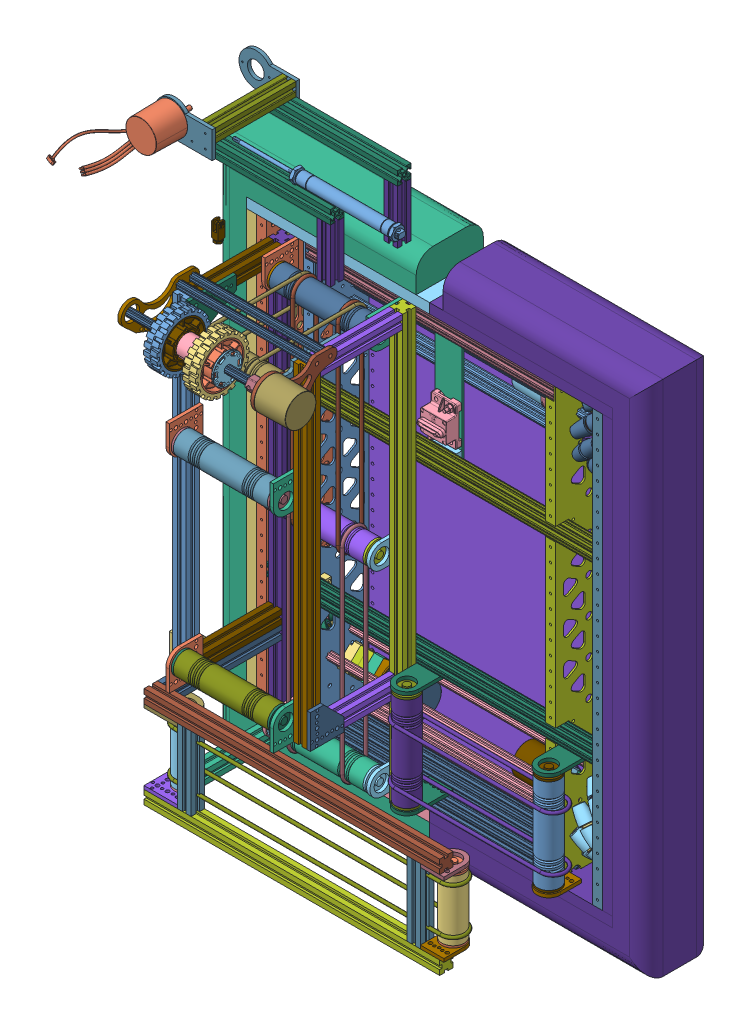
SolidWorks assembly Robot 2020, configuration Default. Lengths in mm. (continued)
Components (placement in the parent): (continued)
- Robot 2020(2)^Robot 2020-1: Robot 2020(2)^Robot 2020 [Default] at origin size (819.15 992.53 549) (virtual) (continued)
  - Fame 2020^Robot 2020(2)_Robot 2020-1: Fame 2020^Robot 2020(2)_Robot 2020 [Default] at origin size (819.15 977.9 171.99) (virtual) (continued)
    - Left Wheel Assembly v4(Mirror) (2)^Fame 2020_Robot 2020(2)_Robot 2020-1: Left Wheel Assembly v4(Mirror) (2)^Fame 2020_Robot 2020(2)_Robot 2020 [Default] at (500 0 0) x (1 0 0) z (0 0 -1) size (65.82 166.11 165.01) (virtual) (continued)
      - 6_Mecanum_Wheel_Left_217-2799 v1(Mirror) (2)^Left Wheel Assembly v4(Mirror) (2)_Fame 2020_Robot 2020(2)_Robot 2020-1: 6_Mecanum_Wheel_Left_217-2799 v1(Mirror) (2)^Left Wheel Assembly v4(Mirror) (2)_Fame 2020_Robot 2020(2)_Robot 2020 [Default] x (0 0 -1) z (1 0 0) size (165.01 166.11 65.82) (virtual) (continued)
        - 217-2586-007 Rev1(Mirror) (2)^6_Mecanum_Wheel_Left_217-2799 v1(Mirror) (2)_Left Wheel Assembly v4(Mirror) (2)_Fame 2020_Robot 2020(2)_Robot 2020-10: 217-2586-007 Rev1(Mirror) (2)^6_Mecanum_Wheel_Left_217-2799 v1(Mirror) (2)_Left Wheel Assembly v4(Mirror) (2)_Fame 2020_Robot 2020(2)_Robot 2020 [Default] at (23.6484 -378.9904 -227.6598) x (0.698401 -0.110616 -0.707107) z (0.159162 0.987249 0.002763) size (61.72 5 5) (virtual)
        - 217-2586-008 Rev1(Mirror) (2)^6_Mecanum_Wheel_Left_217-2799 v1(Mirror) (2)_Left Wheel Assembly v4(Mirror) (2)_Fame 2020_Robot 2020(2)_Robot 2020-1: 217-2586-008 Rev1(Mirror) (2)^6_Mecanum_Wheel_Left_217-2799 v1(Mirror) (2)_Left Wheel Assembly v4(Mirror) (2)_Fame 2020_Robot 2020(2)_Robot 2020 [Default] at (53.3583 -330.4692 -227.5328) x (0.544639 0.838671 0) z (0 0 -1) size (7.33 6.35 31.75) (virtual)
        - 217-2586-008 Rev1(Mirror) (2)^6_Mecanum_Wheel_Left_217-2799 v1(Mirror) (2)_Left Wheel Assembly v4(Mirror) (2)_Fame 2020_Robot 2020(2)_Robot 2020-2: 217-2586-008 Rev1(Mirror) (2)^6_Mecanum_Wheel_Left_217-2799 v1(Mirror) (2)_Left Wheel Assembly v4(Mirror) (2)_Fame 2020_Robot 2020(2)_Robot 2020 [Default] at (32.1413 -341.2799 -227.5328) x (0.99863 -0.052336 0) z (0 0 -1) size (7.33 6.35 31.75) (virtual)
        - 217-2586-008 Rev1(Mirror) (2)^6_Mecanum_Wheel_Left_217-2799 v1(Mirror) (2)_Left Wheel Assembly v4(Mirror) (2)_Fame 2020_Robot 2020(2)_Robot 2020-3: 217-2586-008 Rev1(Mirror) (2)^6_Mecanum_Wheel_Left_217-2799 v1(Mirror) (2)_Left Wheel Assembly v4(Mirror) (2)_Fame 2020_Robot 2020(2)_Robot 2020 [Default] at (12.1704 -328.3106 -227.5328) x (0.45399 -0.891007 0) z (0 0 -1) size (7.33 6.35 31.75) (virtual)
        - 217-2586-008 Rev1(Mirror) (2)^6_Mecanum_Wheel_Left_217-2799 v1(Mirror) (2)_Left Wheel Assembly v4(Mirror) (2)_Fame 2020_Robot 2020(2)_Robot 2020-4: 217-2586-008 Rev1(Mirror) (2)^6_Mecanum_Wheel_Left_217-2799 v1(Mirror) (2)_Left Wheel Assembly v4(Mirror) (2)_Fame 2020_Robot 2020(2)_Robot 2020 [Default] at (13.4167 -304.5308 -227.5328) x (-0.544639 -0.838671 0) z (0 0 -1) size (7.33 6.35 31.75) (virtual)
        - 217-2586-008 Rev1(Mirror) (2)^6_Mecanum_Wheel_Left_217-2799 v1(Mirror) (2)_Left Wheel Assembly v4(Mirror) (2)_Fame 2020_Robot 2020(2)_Robot 2020-5: 217-2586-008 Rev1(Mirror) (2)^6_Mecanum_Wheel_Left_217-2799 v1(Mirror) (2)_Left Wheel Assembly v4(Mirror) (2)_Fame 2020_Robot 2020(2)_Robot 2020 [Default] at (34.6337 -293.7201 -227.5328) x (-0.99863 0.052336 0) z (0 0 -1) size (7.33 6.35 31.75) (virtual)
        - 217-2586-008 Rev1(Mirror) (2)^6_Mecanum_Wheel_Left_217-2799 v1(Mirror) (2)_Left Wheel Assembly v4(Mirror) (2)_Fame 2020_Robot 2020(2)_Robot 2020-6: 217-2586-008 Rev1(Mirror) (2)^6_Mecanum_Wheel_Left_217-2799 v1(Mirror) (2)_Left Wheel Assembly v4(Mirror) (2)_Fame 2020_Robot 2020(2)_Robot 2020 [Default] at (54.6046 -306.6894 -227.5328) x (-0.45399 0.891007 0) z (0 0 -1) size (7.33 6.35 31.75) (virtual)
        - NUT-832-NYLOCK(Mirror) (2)^6_Mecanum_Wheel_Left_217-2799 v1(Mirror) (2)_Left Wheel Assembly v4(Mirror) (2)_Fame 2020_Robot 2020(2)_Robot 2020-1: NUT-832-NYLOCK(Mirror) (2)^6_Mecanum_Wheel_Left_217-2799 v1(Mirror) (2)_Left Wheel Assembly v4(Mirror) (2)_Fame 2020_Robot 2020(2)_Robot 2020 [Default] at (6.1639 -290.2764 -241.3161) x (0.258819 -0.965926 0) z (0.965926 0.258819 0) size (9.37 5.86 8.12) (virtual)
        - NUT-832-NYLOCK(Mirror) (2)^6_Mecanum_Wheel_Left_217-2799 v1(Mirror) (2)_Left Wheel Assembly v4(Mirror) (2)_Fame 2020_Robot 2020(2)_Robot 2020-2: NUT-832-NYLOCK(Mirror) (2)^6_Mecanum_Wheel_Left_217-2799 v1(Mirror) (2)_Left Wheel Assembly v4(Mirror) (2)_Fame 2020_Robot 2020(2)_Robot 2020 [Default] at (-0.9163 -334.9786 -241.3161) x (0.99863 -0.052336 0) z (0.052336 0.99863 0) size (9.37 5.86 8.12) (virtual)
        - NUT-832-NYLOCK(Mirror) (2)^6_Mecanum_Wheel_Left_217-2799 v1(Mirror) (2)_Left Wheel Assembly v4(Mirror) (2)_Fame 2020_Robot 2020(2)_Robot 2020-3: NUT-832-NYLOCK(Mirror) (2)^6_Mecanum_Wheel_Left_217-2799 v1(Mirror) (2)_Left Wheel Assembly v4(Mirror) (2)_Fame 2020_Robot 2020(2)_Robot 2020 [Default] at (39.4102 -355.526 -241.3161) x (0.358368 0.93358 0) z (-0.93358 0.358368 0) size (9.37 5.86 8.12) (virtual)
        - NUT-832-NYLOCK(Mirror) (2)^6_Mecanum_Wheel_Left_217-2799 v1(Mirror) (2)_Left Wheel Assembly v4(Mirror) (2)_Fame 2020_Robot 2020(2)_Robot 2020-4: NUT-832-NYLOCK(Mirror) (2)^6_Mecanum_Wheel_Left_217-2799 v1(Mirror) (2)_Left Wheel Assembly v4(Mirror) (2)_Fame 2020_Robot 2020(2)_Robot 2020 [Default] at (71.4135 -323.5227 -241.3161) x (-0.777146 0.62932 0) z (-0.62932 -0.777146 0) size (9.37 5.86 8.12) (virtual)
        - NUT-832-NYLOCK(Mirror) (2)^6_Mecanum_Wheel_Left_217-2799 v1(Mirror) (2)_Left Wheel Assembly v4(Mirror) (2)_Fame 2020_Robot 2020(2)_Robot 2020-5: NUT-832-NYLOCK(Mirror) (2)^6_Mecanum_Wheel_Left_217-2799 v1(Mirror) (2)_Left Wheel Assembly v4(Mirror) (2)_Fame 2020_Robot 2020(2)_Robot 2020 [Default] at (50.8661 -283.1962 -241.3161) x (-0.838671 -0.544639 0) z (0.544639 -0.838671 0) size (9.37 5.86 8.12) (virtual)
        - SCREW-832-1250(Mirror) (2)^6_Mecanum_Wheel_Left_217-2799 v1(Mirror) (2)_Left Wheel Assembly v4(Mirror) (2)_Fame 2020_Robot 2020(2)_Robot 2020-1: SCREW-832-1250(Mirror) (2)^6_Mecanum_Wheel_Left_217-2799 v1(Mirror) (2)_Left Wheel Assembly v4(Mirror) (2)_Fame 2020_Robot 2020(2)_Robot 2020 [Default] at (6.1639 -290.2764 -212.75) x (0 0 -1) z (0.394243 -0.919006 0) size (33.96 7.92 7.92) (virtual)
        - SCREW-832-1250(Mirror) (2)^6_Mecanum_Wheel_Left_217-2799 v1(Mirror) (2)_Left Wheel Assembly v4(Mirror) (2)_Fame 2020_Robot 2020(2)_Robot 2020-2: SCREW-832-1250(Mirror) (2)^6_Mecanum_Wheel_Left_217-2799 v1(Mirror) (2)_Left Wheel Assembly v4(Mirror) (2)_Fame 2020_Robot 2020(2)_Robot 2020 [Default] at (-0.9163 -334.9786 -212.75) x (0 0 -1) z (0.995855 0.090959 0) size (33.96 7.92 7.92) (virtual)
        - SCREW-832-1250(Mirror) (2)^6_Mecanum_Wheel_Left_217-2799 v1(Mirror) (2)_Left Wheel Assembly v4(Mirror) (2)_Fame 2020_Robot 2020(2)_Robot 2020-3: SCREW-832-1250(Mirror) (2)^6_Mecanum_Wheel_Left_217-2799 v1(Mirror) (2)_Left Wheel Assembly v4(Mirror) (2)_Fame 2020_Robot 2020(2)_Robot 2020 [Default] at (39.4102 -355.526 -212.75) x (0 0 -1) z (0.221229 0.975222 0) size (33.96 7.92 7.92) (virtual)
        - SCREW-832-1250(Mirror) (2)^6_Mecanum_Wheel_Left_217-2799 v1(Mirror) (2)_Left Wheel Assembly v4(Mirror) (2)_Fame 2020_Robot 2020(2)_Robot 2020-4: SCREW-832-1250(Mirror) (2)^6_Mecanum_Wheel_Left_217-2799 v1(Mirror) (2)_Left Wheel Assembly v4(Mirror) (2)_Fame 2020_Robot 2020(2)_Robot 2020 [Default] at (71.4135 -323.5227 -212.75) x (0 0 -1) z (-0.859128 0.511761 0) size (33.96 7.92 7.92) (virtual)
        - SCREW-832-1250(Mirror) (2)^6_Mecanum_Wheel_Left_217-2799 v1(Mirror) (2)_Left Wheel Assembly v4(Mirror) (2)_Fame 2020_Robot 2020(2)_Robot 2020-5: SCREW-832-1250(Mirror) (2)^6_Mecanum_Wheel_Left_217-2799 v1(Mirror) (2)_Left Wheel Assembly v4(Mirror) (2)_Fame 2020_Robot 2020(2)_Robot 2020 [Default] at (50.8661 -283.1962 -212.75) x (0 0 -1) z (-0.752199 -0.658936 0) size (33.96 7.92 7.92) (virtual)
        - 217-2586-005 Rev2(Mirror) (2)^6_Mecanum_Wheel_Left_217-2799 v1(Mirror) (2)_Left Wheel Assembly v4(Mirror) (2)_Fame 2020_Robot 2020(2)_Robot 2020-1: 217-2586-005 Rev2(Mirror) (2)^6_Mecanum_Wheel_Left_217-2799 v1(Mirror) (2)_Left Wheel Assembly v4(Mirror) (2)_Fame 2020_Robot 2020(2)_Robot 2020 [Default] at (-6.1597 -365.9972 -233.9884) x (-0.5 0.5 0.707107) z (-0.146447 -0.853553 0.5) size (8.5 8 8) (virtual)
        - 217-2586-005 Rev2(Mirror) (2)^6_Mecanum_Wheel_Left_217-2799 v1(Mirror) (2)_Left Wheel Assembly v4(Mirror) (2)_Fame 2020_Robot 2020(2)_Robot 2020-2: 217-2586-005 Rev2(Mirror) (2)^6_Mecanum_Wheel_Left_217-2799 v1(Mirror) (2)_Left Wheel Assembly v4(Mirror) (2)_Fame 2020_Robot 2020(2)_Robot 2020 [Default] at (-15.1097 -357.0472 -221.3312) x (-0.5 0.5 0.707107) z (-0.146447 -0.853553 0.5) size (8.5 8 8) (virtual)
        - 217-2586-005 Rev2(Mirror) (2)^6_Mecanum_Wheel_Left_217-2799 v1(Mirror) (2)_Left Wheel Assembly v4(Mirror) (2)_Fame 2020_Robot 2020(2)_Robot 2020-3: 217-2586-005 Rev2(Mirror) (2)^6_Mecanum_Wheel_Left_217-2799 v1(Mirror) (2)_Left Wheel Assembly v4(Mirror) (2)_Fame 2020_Robot 2020(2)_Robot 2020 [Default] at (-29.0929 -320.9884 -221.3312) x (-0.110616 0.698401 0.707107) z (-0.620184 -0.60446 0.5) size (8.5 8 8) (virtual)
        - 217-2586-005 Rev2(Mirror) (2)^6_Mecanum_Wheel_Left_217-2799 v1(Mirror) (2)_Left Wheel Assembly v4(Mirror) (2)_Fame 2020_Robot 2020(2)_Robot 2020-4: 217-2586-005 Rev2(Mirror) (2)^6_Mecanum_Wheel_Left_217-2799 v1(Mirror) (2)_Left Wheel Assembly v4(Mirror) (2)_Fame 2020_Robot 2020(2)_Robot 2020 [Default] at (-19.2106 -283.5972 -221.3312) x (0.32102 0.630037 0.707107) z (-0.857032 -0.124484 0.5) size (8.5 8 8) (virtual)
        - 217-2586-005 Rev2(Mirror) (2)^6_Mecanum_Wheel_Left_217-2799 v1(Mirror) (2)_Left Wheel Assembly v4(Mirror) (2)_Fame 2020_Robot 2020(2)_Robot 2020-5: 217-2586-005 Rev2(Mirror) (2)^6_Mecanum_Wheel_Left_217-2799 v1(Mirror) (2)_Left Wheel Assembly v4(Mirror) (2)_Fame 2020_Robot 2020(2)_Robot 2020 [Default] at (10.7623 -259.1556 -221.3312) x (0.630037 0.32102 0.707107) z (-0.766523 0.403042 0.5) size (8.5 8 8) (virtual)
        - 217-2586-005 Rev2(Mirror) (2)^6_Mecanum_Wheel_Left_217-2799 v1(Mirror) (2)_Left Wheel Assembly v4(Mirror) (2)_Fame 2020_Robot 2020(2)_Robot 2020-6: 217-2586-005 Rev2(Mirror) (2)^6_Mecanum_Wheel_Left_217-2799 v1(Mirror) (2)_Left Wheel Assembly v4(Mirror) (2)_Fame 2020_Robot 2020(2)_Robot 2020 [Default] at (49.3773 -256.9997 -221.3312) x (0.698401 -0.110616 0.707107) z (-0.383228 0.776618 0.5) size (8.5 8 8) (virtual)
        - 217-2586-005 Rev2(Mirror) (2)^6_Mecanum_Wheel_Left_217-2799 v1(Mirror) (2)_Left Wheel Assembly v4(Mirror) (2)_Fame 2020_Robot 2020(2)_Robot 2020-7: 217-2586-005 Rev2(Mirror) (2)^6_Mecanum_Wheel_Left_217-2799 v1(Mirror) (2)_Left Wheel Assembly v4(Mirror) (2)_Fame 2020_Robot 2020(2)_Robot 2020 [Default] at (81.8847 -277.9528 -221.3312) x (0.5 -0.5 0.707107) z (0.146447 0.853553 0.5) size (8.5 8 8) (virtual)
        - 217-2586-005 Rev2(Mirror) (2)^6_Mecanum_Wheel_Left_217-2799 v1(Mirror) (2)_Left Wheel Assembly v4(Mirror) (2)_Fame 2020_Robot 2020(2)_Robot 2020-8: 217-2586-005 Rev2(Mirror) (2)^6_Mecanum_Wheel_Left_217-2799 v1(Mirror) (2)_Left Wheel Assembly v4(Mirror) (2)_Fame 2020_Robot 2020(2)_Robot 2020 [Default] at (95.8679 -314.0116 -221.3312) x (0.110616 -0.698401 0.707107) z (0.620184 0.60446 0.5) size (8.5 8 8) (virtual)
        - 217-2586-005 Rev2(Mirror) (2)^6_Mecanum_Wheel_Left_217-2799 v1(Mirror) (2)_Left Wheel Assembly v4(Mirror) (2)_Fame 2020_Robot 2020(2)_Robot 2020-9: 217-2586-005 Rev2(Mirror) (2)^6_Mecanum_Wheel_Left_217-2799 v1(Mirror) (2)_Left Wheel Assembly v4(Mirror) (2)_Fame 2020_Robot 2020(2)_Robot 2020 [Default] at (85.9856 -351.4028 -221.3312) x (-0.32102 -0.630037 0.707107) z (0.857032 0.124484 0.5) size (8.5 8 8) (virtual)
        - 217-2586-005 Rev2(Mirror) (2)^6_Mecanum_Wheel_Left_217-2799 v1(Mirror) (2)_Left Wheel Assembly v4(Mirror) (2)_Fame 2020_Robot 2020(2)_Robot 2020-10: 217-2586-005 Rev2(Mirror) (2)^6_Mecanum_Wheel_Left_217-2799 v1(Mirror) (2)_Left Wheel Assembly v4(Mirror) (2)_Fame 2020_Robot 2020(2)_Robot 2020 [Default] at (56.0127 -375.8444 -221.3312) x (-0.630037 -0.32102 0.707107) z (0.766523 -0.403042 0.5) size (8.5 8 8) (virtual)
        - 217-2586-005 Rev2(Mirror) (2)^6_Mecanum_Wheel_Left_217-2799 v1(Mirror) (2)_Left Wheel Assembly v4(Mirror) (2)_Fame 2020_Robot 2020(2)_Robot 2020-11: 217-2586-005 Rev2(Mirror) (2)^6_Mecanum_Wheel_Left_217-2799 v1(Mirror) (2)_Left Wheel Assembly v4(Mirror) (2)_Fame 2020_Robot 2020(2)_Robot 2020 [Default] at (17.3977 -378.0003 -221.3312) x (-0.698401 0.110616 0.707107) z (0.383228 -0.776618 0.5) size (8.5 8 8) (virtual)
        - 217-2586-005 Rev2(Mirror) (2)^6_Mecanum_Wheel_Left_217-2799 v1(Mirror) (2)_Left Wheel Assembly v4(Mirror) (2)_Fame 2020_Robot 2020(2)_Robot 2020-12: 217-2586-005 Rev2(Mirror) (2)^6_Mecanum_Wheel_Left_217-2799 v1(Mirror) (2)_Left Wheel Assembly v4(Mirror) (2)_Fame 2020_Robot 2020(2)_Robot 2020 [Default] at (-27.1128 -333.4898 -233.9884) x (-0.110616 0.698401 0.707107) z (-0.620184 -0.60446 0.5) size (8.5 8 8) (virtual)
        - 217-2586-005 Rev2(Mirror) (2)^6_Mecanum_Wheel_Left_217-2799 v1(Mirror) (2)_Left Wheel Assembly v4(Mirror) (2)_Fame 2020_Robot 2020(2)_Robot 2020-13: 217-2586-005 Rev2(Mirror) (2)^6_Mecanum_Wheel_Left_217-2799 v1(Mirror) (2)_Left Wheel Assembly v4(Mirror) (2)_Fame 2020_Robot 2020(2)_Robot 2020 [Default] at (-24.9569 -294.8748 -233.9884) x (0.32102 0.630037 0.707107) z (-0.857032 -0.124484 0.5) size (8.5 8 8) (virtual)
        - 217-2586-005 Rev2(Mirror) (2)^6_Mecanum_Wheel_Left_217-2799 v1(Mirror) (2)_Left Wheel Assembly v4(Mirror) (2)_Fame 2020_Robot 2020(2)_Robot 2020-14: 217-2586-005 Rev2(Mirror) (2)^6_Mecanum_Wheel_Left_217-2799 v1(Mirror) (2)_Left Wheel Assembly v4(Mirror) (2)_Fame 2020_Robot 2020(2)_Robot 2020 [Default] at (-0.5153 -264.9019 -233.9884) x (0.630037 0.32102 0.707107) z (-0.766523 0.403042 0.5) size (8.5 8 8) (virtual)
        - 217-2586-005 Rev2(Mirror) (2)^6_Mecanum_Wheel_Left_217-2799 v1(Mirror) (2)_Left Wheel Assembly v4(Mirror) (2)_Fame 2020_Robot 2020(2)_Robot 2020-15: 217-2586-005 Rev2(Mirror) (2)^6_Mecanum_Wheel_Left_217-2799 v1(Mirror) (2)_Left Wheel Assembly v4(Mirror) (2)_Fame 2020_Robot 2020(2)_Robot 2020 [Default] at (36.8759 -255.0196 -233.9884) x (0.698401 -0.110616 0.707107) z (-0.383228 0.776618 0.5) size (8.5 8 8) (virtual)
        - 217-2586-005 Rev2(Mirror) (2)^6_Mecanum_Wheel_Left_217-2799 v1(Mirror) (2)_Left Wheel Assembly v4(Mirror) (2)_Fame 2020_Robot 2020(2)_Robot 2020-16: 217-2586-005 Rev2(Mirror) (2)^6_Mecanum_Wheel_Left_217-2799 v1(Mirror) (2)_Left Wheel Assembly v4(Mirror) (2)_Fame 2020_Robot 2020(2)_Robot 2020 [Default] at (72.9347 -269.0028 -233.9884) x (0.5 -0.5 0.707107) z (0.146447 0.853553 0.5) size (8.5 8 8) (virtual)
        - 217-2586-005 Rev2(Mirror) (2)^6_Mecanum_Wheel_Left_217-2799 v1(Mirror) (2)_Left Wheel Assembly v4(Mirror) (2)_Fame 2020_Robot 2020(2)_Robot 2020-17: 217-2586-005 Rev2(Mirror) (2)^6_Mecanum_Wheel_Left_217-2799 v1(Mirror) (2)_Left Wheel Assembly v4(Mirror) (2)_Fame 2020_Robot 2020(2)_Robot 2020 [Default] at (93.8878 -301.5102 -233.9884) x (0.110616 -0.698401 0.707107) z (0.620184 0.60446 0.5) size (8.5 8 8) (virtual)
        - 217-2586-005 Rev2(Mirror) (2)^6_Mecanum_Wheel_Left_217-2799 v1(Mirror) (2)_Left Wheel Assembly v4(Mirror) (2)_Fame 2020_Robot 2020(2)_Robot 2020-18: 217-2586-005 Rev2(Mirror) (2)^6_Mecanum_Wheel_Left_217-2799 v1(Mirror) (2)_Left Wheel Assembly v4(Mirror) (2)_Fame 2020_Robot 2020(2)_Robot 2020 [Default] at (91.7319 -340.1252 -233.9884) x (-0.32102 -0.630037 0.707107) z (0.857032 0.124484 0.5) size (8.5 8 8) (virtual)
        - 217-2586-005 Rev2(Mirror) (2)^6_Mecanum_Wheel_Left_217-2799 v1(Mirror) (2)_Left Wheel Assembly v4(Mirror) (2)_Fame 2020_Robot 2020(2)_Robot 2020-19: 217-2586-005 Rev2(Mirror) (2)^6_Mecanum_Wheel_Left_217-2799 v1(Mirror) (2)_Left Wheel Assembly v4(Mirror) (2)_Fame 2020_Robot 2020(2)_Robot 2020 [Default] at (67.2903 -370.0981 -233.9884) x (-0.630037 -0.32102 0.707107) z (0.766523 -0.403042 0.5) size (8.5 8 8) (virtual)
        - 217-2586-005 Rev2(Mirror) (2)^6_Mecanum_Wheel_Left_217-2799 v1(Mirror) (2)_Left Wheel Assembly v4(Mirror) (2)_Fame 2020_Robot 2020(2)_Robot 2020-20: 217-2586-005 Rev2(Mirror) (2)^6_Mecanum_Wheel_Left_217-2799 v1(Mirror) (2)_Left Wheel Assembly v4(Mirror) (2)_Fame 2020_Robot 2020(2)_Robot 2020 [Default] at (29.8991 -379.9804 -233.9884) x (-0.698401 0.110616 0.707107) z (0.383228 -0.776618 0.5) size (8.5 8 8) (virtual)
      - 1_2_Hex_Bore_Aluminum_VersaHub_217-2592 v1(Mirror) (2)^Left Wheel Assembly v4(Mirror) (2)_Fame 2020_Robot 2020(2)_Robot 2020-1: 1_2_Hex_Bore_Aluminum_VersaHub_217-2592 v1(Mirror) (2)^Left Wheel Assembly v4(Mirror) (2)_Fame 2020_Robot 2020(2)_Robot 2020 [Default] at (-239.7248 -317.5 -33.3875) x (-1 0 0) z (0 -0.707107 0.707107) size (12.7 55.88 55.88) (virtual)
    - NEO Gearbox 2-stage Custom v5(Mirror)^Fame 2020_Robot 2020(2)_Robot 2020-1: NEO Gearbox 2-stage Custom v5(Mirror)^Fame 2020_Robot 2020(2)_Robot 2020 [Default] at (0 0 425) x (-1 0 0) z (0 0 -1) size (164.9 90.53 90.53) (virtual)
      - VersaPlanetary_4_1_Gear_Kit_217-2818 v1(Mirror)^NEO Gearbox 2-stage Custom v5(Mirror)_Fame 2020_Robot 2020(2)_Robot 2020-1: VersaPlanetary_4_1_Gear_Kit_217-2818 v1(Mirror)^NEO Gearbox 2-stage Custom v5(Mirror)_Fame 2020_Robot 2020(2)_Robot 2020 [Default] at (-15.25 22.225 0) x (0 -0.707107 -0.707107) z (1 0 0) size (35.49 35.49 17.4) (virtual)
        - 217-2725-001 Rev1_24t Sun(Mirror)^VersaPlanetary_4_1_Gear_Kit_217-2818 v1(Mirror)_NEO Gearbox 2-stage Custom v5(Mirror)_Fame 2020_Robot 2020(2)_Robot 2020-1: 217-2725-001 Rev1_24t Sun(Mirror)^VersaPlanetary_4_1_Gear_Kit_217-2818 v1(Mirror)_NEO Gearbox 2-stage Custom v5(Mirror)_Fame 2020_Robot 2020(2)_Robot 2020 [Default] at (-36.69 -517.1337 209.675) x (0.707107 0.707107 0) z (0 0 1) size (14.4 14.45 12.7) (virtual)
        - 217-2725-002 Rev1_24t Planet(Mirror)^VersaPlanetary_4_1_Gear_Kit_217-2818 v1(Mirror)_NEO Gearbox 2-stage Custom v5(Mirror)_Fame 2020_Robot 2020(2)_Robot 2020-1: 217-2725-002 Rev1_24t Planet(Mirror)^VersaPlanetary_4_1_Gear_Kit_217-2818 v1(Mirror)_NEO Gearbox 2-stage Custom v5(Mirror)_Fame 2020_Robot 2020(2)_Robot 2020 [Default] at (-45.2382 -525.6819 212.025) x (-0.793353 0.608761 0) z (0 0 -1) size (13.12 13.1 8) (virtual)
        - 217-2725-002 Rev1_24t Planet(Mirror)^VersaPlanetary_4_1_Gear_Kit_217-2818 v1(Mirror)_NEO Gearbox 2-stage Custom v5(Mirror)_Fame 2020_Robot 2020(2)_Robot 2020-2: 217-2725-002 Rev1_24t Planet(Mirror)^VersaPlanetary_4_1_Gear_Kit_217-2818 v1(Mirror)_NEO Gearbox 2-stage Custom v5(Mirror)_Fame 2020_Robot 2020(2)_Robot 2020 [Default] at (-28.1418 -525.6819 212.025) x (-0.608761 -0.793353 0) z (0 0 -1) size (13.12 13.1 8) (virtual)
        - 217-2725-002 Rev1_24t Planet(Mirror)^VersaPlanetary_4_1_Gear_Kit_217-2818 v1(Mirror)_NEO Gearbox 2-stage Custom v5(Mirror)_Fame 2020_Robot 2020(2)_Robot 2020-3: 217-2725-002 Rev1_24t Planet(Mirror)^VersaPlanetary_4_1_Gear_Kit_217-2818 v1(Mirror)_NEO Gearbox 2-stage Custom v5(Mirror)_Fame 2020_Robot 2020(2)_Robot 2020 [Default] at (-28.1418 -508.5855 212.025) x (0.793353 -0.608761 0) z (0 0 -1) size (13.12 13.1 8) (virtual)
        - 217-2725-002 Rev1_24t Planet(Mirror)^VersaPlanetary_4_1_Gear_Kit_217-2818 v1(Mirror)_NEO Gearbox 2-stage Custom v5(Mirror)_Fame 2020_Robot 2020(2)_Robot 2020-4: 217-2725-002 Rev1_24t Planet(Mirror)^VersaPlanetary_4_1_Gear_Kit_217-2818 v1(Mirror)_NEO Gearbox 2-stage Custom v5(Mirror)_Fame 2020_Robot 2020(2)_Robot 2020 [Default] at (-45.2382 -508.5855 212.025) x (0.608761 0.793353 0) z (0 0 -1) size (13.12 13.1 8) (virtual)
        - 217-2724-002 Rev1(Mirror)^VersaPlanetary_4_1_Gear_Kit_217-2818 v1(Mirror)_NEO Gearbox 2-stage Custom v5(Mirror)_Fame 2020_Robot 2020(2)_Robot 2020-1: 217-2724-002 Rev1(Mirror)^VersaPlanetary_4_1_Gear_Kit_217-2818 v1(Mirror)_NEO Gearbox 2-stage Custom v5(Mirror)_Fame 2020_Robot 2020(2)_Robot 2020 [Default] at (-36.69 -517.1337 218.375) x (1 0 0) z (0 0 -1) size (34.7 34.7 4.7) (virtual)
        - 217-2625-010 Rev1(Mirror)^VersaPlanetary_4_1_Gear_Kit_217-2818 v1(Mirror)_NEO Gearbox 2-stage Custom v5(Mirror)_Fame 2020_Robot 2020(2)_Robot 2020-1: 217-2625-010 Rev1(Mirror)^VersaPlanetary_4_1_Gear_Kit_217-2818 v1(Mirror)_NEO Gearbox 2-stage Custom v5(Mirror)_Fame 2020_Robot 2020(2)_Robot 2020 [Default] at (-45.2382 -525.6819 214.725) x (0.854322 0.519745 0) z (0 0 1) size (4 4 12) (virtual)
        - 217-2625-010 Rev1(Mirror)^VersaPlanetary_4_1_Gear_Kit_217-2818 v1(Mirror)_NEO Gearbox 2-stage Custom v5(Mirror)_Fame 2020_Robot 2020(2)_Robot 2020-2: 217-2625-010 Rev1(Mirror)^VersaPlanetary_4_1_Gear_Kit_217-2818 v1(Mirror)_NEO Gearbox 2-stage Custom v5(Mirror)_Fame 2020_Robot 2020(2)_Robot 2020 [Default] at (-28.1418 -525.6819 214.725) x (-0.519745 0.854322 0) z (0 0 1) size (4 4 12) (virtual)
        - 217-2625-010 Rev1(Mirror)^VersaPlanetary_4_1_Gear_Kit_217-2818 v1(Mirror)_NEO Gearbox 2-stage Custom v5(Mirror)_Fame 2020_Robot 2020(2)_Robot 2020-3: 217-2625-010 Rev1(Mirror)^VersaPlanetary_4_1_Gear_Kit_217-2818 v1(Mirror)_NEO Gearbox 2-stage Custom v5(Mirror)_Fame 2020_Robot 2020(2)_Robot 2020 [Default] at (-28.1418 -508.5855 214.725) x (-0.854322 -0.519745 0) z (0 0 1) size (4 4 12) (virtual)
        - 217-2625-010 Rev1(Mirror)^VersaPlanetary_4_1_Gear_Kit_217-2818 v1(Mirror)_NEO Gearbox 2-stage Custom v5(Mirror)_Fame 2020_Robot 2020(2)_Robot 2020-4: 217-2625-010 Rev1(Mirror)^VersaPlanetary_4_1_Gear_Kit_217-2818 v1(Mirror)_NEO Gearbox 2-stage Custom v5(Mirror)_Fame 2020_Robot 2020(2)_Robot 2020 [Default] at (-45.2382 -508.5855 214.725) x (0.519745 -0.854322 0) z (0 0 1) size (4 4 12) (virtual)
      - 217-2625-026 Rev1(Mirror)^NEO Gearbox 2-stage Custom v5(Mirror)_Fame 2020_Robot 2020(2)_Robot 2020-1: 217-2625-026 Rev1(Mirror)^NEO Gearbox 2-stage Custom v5(Mirror)_Fame 2020_Robot 2020(2)_Robot 2020 [Default] at (211.875 -317.5 391.6125) x (0 -0.707107 -0.707107) z (1 0 0) size (44.45 42 18.12) (virtual)
      - 217-2742-001 Rev4(Mirror)^NEO Gearbox 2-stage Custom v5(Mirror)_Fame 2020_Robot 2020(2)_Robot 2020-1: 217-2742-001 Rev4(Mirror)^NEO Gearbox 2-stage Custom v5(Mirror)_Fame 2020_Robot 2020(2)_Robot 2020 [Default] at (218.5752 -317.5 391.6125) x (1 0 0) z (0 -0.63857 0.769564) size (7 28 28) (virtual)
      - 217-2742-001 Rev4(Mirror)^NEO Gearbox 2-stage Custom v5(Mirror)_Fame 2020_Robot 2020(2)_Robot 2020-2: 217-2742-001 Rev4(Mirror)^NEO Gearbox 2-stage Custom v5(Mirror)_Fame 2020_Robot 2020(2)_Robot 2020 [Default] at (226.5752 -317.5 391.6125) x (1 0 0) z (0 -0.707107 0.707107) size (7 28 28) (virtual)
      - 217-2625-017 Rev1_9714K61(Mirror)^NEO Gearbox 2-stage Custom v5(Mirror)_Fame 2020_Robot 2020(2)_Robot 2020-1: 217-2625-017 Rev1_9714K61(Mirror)^NEO Gearbox 2-stage Custom v5(Mirror)_Fame 2020_Robot 2020(2)_Robot 2020 [Default] at (225.795 -317.6887 391.9075) x (0 0.983393 -0.181491) z (0 0.181491 0.983393) size (28.51 4.98 27.43) (virtual)
      - 217-2625-025 Rev1(Mirror)^NEO Gearbox 2-stage Custom v5(Mirror)_Fame 2020_Robot 2020(2)_Robot 2020-1: 217-2625-025 Rev1(Mirror)^NEO Gearbox 2-stage Custom v5(Mirror)_Fame 2020_Robot 2020(2)_Robot 2020 [Default] at (182.475 -317.5 391.6125) x (0 -0.707107 -0.707107) z (1 0 0) size (44.45 42 18) (virtual)
      - 217-2816-001 Rev1(Mirror)^NEO Gearbox 2-stage Custom v5(Mirror)_Fame 2020_Robot 2020(2)_Robot 2020-1: 217-2816-001 Rev1(Mirror)^NEO Gearbox 2-stage Custom v5(Mirror)_Fame 2020_Robot 2020(2)_Robot 2020 [Default] at (212.025 -317.5 391.6125) x (0 -0.707107 -0.707107) z (-1 0 0) size (42 42 14.5) (virtual)
      - 217-2816-001 Rev1(Mirror)^NEO Gearbox 2-stage Custom v5(Mirror)_Fame 2020_Robot 2020(2)_Robot 2020-2: 217-2816-001 Rev1(Mirror)^NEO Gearbox 2-stage Custom v5(Mirror)_Fame 2020_Robot 2020(2)_Robot 2020 [Default] at (199.325 -317.5 391.6125) x (0 -0.707107 -0.707107) z (-1 0 0) size (42 42 14.5) (virtual)
      - 217-4649-001 Rev1(Mirror)^NEO Gearbox 2-stage Custom v5(Mirror)_Fame 2020_Robot 2020(2)_Robot 2020-1: 217-4649-001 Rev1(Mirror)^NEO Gearbox 2-stage Custom v5(Mirror)_Fame 2020_Robot 2020(2)_Robot 2020 [Default] at (185.629 -317.5 391.6125) x (0 -0.707107 -0.707107) z (-1 0 0) size (18 18 13) (virtual)
      - VersaPlanetary_CIM_Adapter_217-4018 v1(Mirror)^NEO Gearbox 2-stage Custom v5(Mirror)_Fame 2020_Robot 2020(2)_Robot 2020-1: VersaPlanetary_CIM_Adapter_217-4018 v1(Mirror)^NEO Gearbox 2-stage Custom v5(Mirror)_Fame 2020_Robot 2020(2)_Robot 2020 [Default] at (165.15 -317.5 391.6125) x (0 -0.707107 -0.707107) z (0 -0.707107 0.707107) size (64.01 21.55 64.01) (virtual)
      - NEO Motor REV-21-1650 v2(Mirror)^NEO Gearbox 2-stage Custom v5(Mirror)_Fame 2020_Robot 2020(2)_Robot 2020-1: NEO Motor REV-21-1650 v2(Mirror)^NEO Gearbox 2-stage Custom v5(Mirror)_Fame 2020_Robot 2020(2)_Robot 2020 [Default] at (153.625 -317.5 391.6125) x (0 -0.707107 0.707107) z (-1 0 0) size (61.14 61.02 93.25) (virtual)
      - 3_1 Output Shaft Custom v6(Mirror)^NEO Gearbox 2-stage Custom v5(Mirror)_Fame 2020_Robot 2020(2)_Robot 2020-1: 3_1 Output Shaft Custom v6(Mirror)^NEO Gearbox 2-stage Custom v5(Mirror)_Fame 2020_Robot 2020(2)_Robot 2020 [Default] at (211.3752 -317.5 391.6125) x (1 0 0) z (0 -0.707107 0.707107) size (48.9 34.7 34.7) (virtual)
    - Left Wheel Assembly v4(Mirror)^Fame 2020_Robot 2020(2)_Robot 2020-1: Left Wheel Assembly v4(Mirror)^Fame 2020_Robot 2020(2)_Robot 2020 [Default] at (-500 0 0) x (-1 0 0) z (0 0 -1) size (65.82 166.11 165.01) (virtual)
      - 6_Mecanum_Wheel_Left_217-2799 v1(Mirror)^Left Wheel Assembly v4(Mirror)_Fame 2020_Robot 2020(2)_Robot 2020-1: 6_Mecanum_Wheel_Left_217-2799 v1(Mirror)^Left Wheel Assembly v4(Mirror)_Fame 2020_Robot 2020(2)_Robot 2020 [Default] x (0 0 -1) z (1 0 0) size (165.01 166.11 65.82) (virtual)
        - 217-2799-001 Rev1(Mirror)^6_Mecanum_Wheel_Left_217-2799 v1(Mirror)_Left Wheel Assembly v4(Mirror)_Fame 2020_Robot 2020(2)_Robot 2020-1: 217-2799-001 Rev1(Mirror)^6_Mecanum_Wheel_Left_217-2799 v1(Mirror)_Left Wheel Assembly v4(Mirror)_Fame 2020_Robot 2020(2)_Robot 2020 [Default] at (33.3875 -317.5 -234.0098) x (0.707107 0.707107 0) z (0 0 1) size (95.78 100.46 28.55) (virtual)
        - 217-2799-001 Rev1(Mirror)^6_Mecanum_Wheel_Left_217-2799 v1(Mirror)_Left Wheel Assembly v4(Mirror)_Fame 2020_Robot 2020(2)_Robot 2020-2: 217-2799-001 Rev1(Mirror)^6_Mecanum_Wheel_Left_217-2799 v1(Mirror)_Left Wheel Assembly v4(Mirror)_Fame 2020_Robot 2020(2)_Robot 2020 [Default] at (33.3875 -317.5 -221.3098) x (-0.987688 -0.156434 0) z (0 0 -1) size (95.78 100.46 28.55) (virtual)
        - 217-2799-002 Rev1(Mirror)^6_Mecanum_Wheel_Left_217-2799 v1(Mirror)_Left Wheel Assembly v4(Mirror)_Fame 2020_Robot 2020(2)_Robot 2020-1: 217-2799-002 Rev1(Mirror)^6_Mecanum_Wheel_Left_217-2799 v1(Mirror)_Left Wheel Assembly v4(Mirror)_Fame 2020_Robot 2020(2)_Robot 2020 [Default] at (4.057 -346.8305 -227.6598) x (-0.707107 0.707107 0) z (0.707107 0.707107 0) size (26.84 25.39 30.1) (virtual)
        - 217-2799-002 Rev1(Mirror)^6_Mecanum_Wheel_Left_217-2799 v1(Mirror)_Left Wheel Assembly v4(Mirror)_Fame 2020_Robot 2020(2)_Robot 2020-2: 217-2799-002 Rev1(Mirror)^6_Mecanum_Wheel_Left_217-2799 v1(Mirror)_Left Wheel Assembly v4(Mirror)_Fame 2020_Robot 2020(2)_Robot 2020 [Default] at (-7.5815 -323.9888 -227.6598) x (-0.156434 0.987688 0) z (0.987688 0.156434 0) size (26.84 25.39 30.1) (virtual)
        - 217-2799-002 Rev1(Mirror)^6_Mecanum_Wheel_Left_217-2799 v1(Mirror)_Left Wheel Assembly v4(Mirror)_Fame 2020_Robot 2020(2)_Robot 2020-3: 217-2799-002 Rev1(Mirror)^6_Mecanum_Wheel_Left_217-2799 v1(Mirror)_Left Wheel Assembly v4(Mirror)_Fame 2020_Robot 2020(2)_Robot 2020 [Default] at (-3.5711 -298.6686 -227.6598) x (0.45399 0.891007 0) z (0.891007 -0.45399 0) size (26.84 25.39 30.1) (virtual)
        - 217-2799-002 Rev1(Mirror)^6_Mecanum_Wheel_Left_217-2799 v1(Mirror)_Left Wheel Assembly v4(Mirror)_Fame 2020_Robot 2020(2)_Robot 2020-4: 217-2799-002 Rev1(Mirror)^6_Mecanum_Wheel_Left_217-2799 v1(Mirror)_Left Wheel Assembly v4(Mirror)_Fame 2020_Robot 2020(2)_Robot 2020 [Default] at (14.5561 -280.5414 -227.6598) x (0.891007 0.45399 0) z (0.45399 -0.891007 0) size (26.84 25.39 30.1) (virtual)
        - 217-2799-002 Rev1(Mirror)^6_Mecanum_Wheel_Left_217-2799 v1(Mirror)_Left Wheel Assembly v4(Mirror)_Fame 2020_Robot 2020(2)_Robot 2020-5: 217-2799-002 Rev1(Mirror)^6_Mecanum_Wheel_Left_217-2799 v1(Mirror)_Left Wheel Assembly v4(Mirror)_Fame 2020_Robot 2020(2)_Robot 2020 [Default] at (39.8763 -276.531 -227.6598) x (0.987688 -0.156434 0) z (-0.156434 -0.987688 0) size (26.84 25.39 30.1) (virtual)
        - 217-2799-002 Rev1(Mirror)^6_Mecanum_Wheel_Left_217-2799 v1(Mirror)_Left Wheel Assembly v4(Mirror)_Fame 2020_Robot 2020(2)_Robot 2020-6: 217-2799-002 Rev1(Mirror)^6_Mecanum_Wheel_Left_217-2799 v1(Mirror)_Left Wheel Assembly v4(Mirror)_Fame 2020_Robot 2020(2)_Robot 2020 [Default] at (62.718 -288.1695 -227.6598) x (0.707107 -0.707107 0) z (-0.707107 -0.707107 0) size (26.84 25.39 30.1) (virtual)
        - 217-2799-002 Rev1(Mirror)^6_Mecanum_Wheel_Left_217-2799 v1(Mirror)_Left Wheel Assembly v4(Mirror)_Fame 2020_Robot 2020(2)_Robot 2020-7: 217-2799-002 Rev1(Mirror)^6_Mecanum_Wheel_Left_217-2799 v1(Mirror)_Left Wheel Assembly v4(Mirror)_Fame 2020_Robot 2020(2)_Robot 2020 [Default] at (74.3565 -311.0112 -227.6598) x (0.156434 -0.987688 0) z (-0.987688 -0.156434 0) size (26.84 25.39 30.1) (virtual)
        - 217-2799-002 Rev1(Mirror)^6_Mecanum_Wheel_Left_217-2799 v1(Mirror)_Left Wheel Assembly v4(Mirror)_Fame 2020_Robot 2020(2)_Robot 2020-8: 217-2799-002 Rev1(Mirror)^6_Mecanum_Wheel_Left_217-2799 v1(Mirror)_Left Wheel Assembly v4(Mirror)_Fame 2020_Robot 2020(2)_Robot 2020 [Default] at (70.3461 -336.3314 -227.6598) x (-0.45399 -0.891007 0) z (-0.891007 0.45399 0) size (26.84 25.39 30.1) (virtual)
        - 217-2799-002 Rev1(Mirror)^6_Mecanum_Wheel_Left_217-2799 v1(Mirror)_Left Wheel Assembly v4(Mirror)_Fame 2020_Robot 2020(2)_Robot 2020-9: 217-2799-002 Rev1(Mirror)^6_Mecanum_Wheel_Left_217-2799 v1(Mirror)_Left Wheel Assembly v4(Mirror)_Fame 2020_Robot 2020(2)_Robot 2020 [Default] at (52.2189 -354.4586 -227.6598) x (-0.891007 -0.45399 0) z (-0.45399 0.891007 0) size (26.84 25.39 30.1) (virtual)
        - 217-2799-002 Rev1(Mirror)^6_Mecanum_Wheel_Left_217-2799 v1(Mirror)_Left Wheel Assembly v4(Mirror)_Fame 2020_Robot 2020(2)_Robot 2020-10: 217-2799-002 Rev1(Mirror)^6_Mecanum_Wheel_Left_217-2799 v1(Mirror)_Left Wheel Assembly v4(Mirror)_Fame 2020_Robot 2020(2)_Robot 2020 [Default] at (26.8987 -358.469 -227.6598) x (-0.987688 0.156434 0) z (0.156434 0.987688 0) size (26.84 25.39 30.1) (virtual)
        - 217-2586-003 Rev2(Mirror)^6_Mecanum_Wheel_Left_217-2799 v1(Mirror)_Left Wheel Assembly v4(Mirror)_Fame 2020_Robot 2020(2)_Robot 2020-1: 217-2586-003 Rev2(Mirror)^6_Mecanum_Wheel_Left_217-2799 v1(Mirror)_Left Wheel Assembly v4(Mirror)_Fame 2020_Robot 2020(2)_Robot 2020 [Default] at (-13.4676 -358.6894 -223.6536) x (0.41944 0.854155 -0.30739) z (0.757674 -0.142894 0.636798) size (19.46 28.57 19.46) (virtual)
        - 217-2586-003 Rev2(Mirror)^6_Mecanum_Wheel_Left_217-2799 v1(Mirror)_Left Wheel Assembly v4(Mirror)_Fame 2020_Robot 2020(2)_Robot 2020-2: 217-2586-003 Rev2(Mirror)^6_Mecanum_Wheel_Left_217-2799 v1(Mirror)_Left Wheel Assembly v4(Mirror)_Fame 2020_Robot 2020(2)_Robot 2020 [Default] at (-7.8019 -364.3551 -231.666) x (0.847342 0.451134 0.280161) z (-0.17892 0.739241 -0.649238) size (19.46 28.57 19.46) (virtual)
        - 217-2586-003 Rev2(Mirror)^6_Mecanum_Wheel_Left_217-2799 v1(Mirror)_Left Wheel Assembly v4(Mirror)_Fame 2020_Robot 2020(2)_Robot 2020-3: 217-2586-003 Rev2(Mirror)^6_Mecanum_Wheel_Left_217-2799 v1(Mirror)_Left Wheel Assembly v4(Mirror)_Fame 2020_Robot 2020(2)_Robot 2020 [Default] at (-27.4761 -331.196 -231.666) x (0.950684 -0.13308 0.280161) z (0.289766 0.703225 -0.649238) size (19.46 28.57 19.46) (virtual)
        - 217-2586-003 Rev2(Mirror)^6_Mecanum_Wheel_Left_217-2799 v1(Mirror)_Left Wheel Assembly v4(Mirror)_Fame 2020_Robot 2020(2)_Robot 2020-4: 217-2586-003 Rev2(Mirror)^6_Mecanum_Wheel_Left_217-2799 v1(Mirror)_Left Wheel Assembly v4(Mirror)_Fame 2020_Robot 2020(2)_Robot 2020 [Default] at (-23.9025 -292.8056 -231.666) x (0.690897 -0.666462 0.280161) z (0.647771 0.398601 -0.649238) size (19.46 28.57 19.46) (virtual)
        - 217-2586-003 Rev2(Mirror)^6_Mecanum_Wheel_Left_217-2799 v1(Mirror)_Left Wheel Assembly v4(Mirror)_Fame 2020_Robot 2020(2)_Robot 2020-5: 217-2586-003 Rev2(Mirror)^6_Mecanum_Wheel_Left_217-2799 v1(Mirror)_Left Wheel Assembly v4(Mirror)_Fame 2020_Robot 2020(2)_Robot 2020 [Default] at (1.5539 -263.8475 -231.666) x (0.167211 -0.945278 0.280161) z (0.75835 -0.058276 -0.649238) size (19.46 28.57 19.46) (virtual)
        - 217-2586-003 Rev2(Mirror)^6_Mecanum_Wheel_Left_217-2799 v1(Mirror)_Left Wheel Assembly v4(Mirror)_Fame 2020_Robot 2020(2)_Robot 2020-6: 217-2586-003 Rev2(Mirror)^6_Mecanum_Wheel_Left_217-2799 v1(Mirror)_Left Wheel Assembly v4(Mirror)_Fame 2020_Robot 2020(2)_Robot 2020 [Default] at (39.1697 -255.3829 -231.666) x (-0.420344 -0.86303 0.280161) z (0.579264 -0.492893 -0.649238) size (19.46 28.57 19.46) (virtual)
        - 217-2586-003 Rev2(Mirror)^6_Mecanum_Wheel_Left_217-2799 v1(Mirror)_Left Wheel Assembly v4(Mirror)_Fame 2020_Robot 2020(2)_Robot 2020-7: 217-2586-003 Rev2(Mirror)^6_Mecanum_Wheel_Left_217-2799 v1(Mirror)_Left Wheel Assembly v4(Mirror)_Fame 2020_Robot 2020(2)_Robot 2020 [Default] at (74.5769 -270.6449 -231.666) x (-0.847342 -0.451134 0.280161) z (0.17892 -0.739241 -0.649238) size (19.46 28.57 19.46) (virtual)
        - 217-2586-003 Rev2(Mirror)^6_Mecanum_Wheel_Left_217-2799 v1(Mirror)_Left Wheel Assembly v4(Mirror)_Fame 2020_Robot 2020(2)_Robot 2020-8: 217-2586-003 Rev2(Mirror)^6_Mecanum_Wheel_Left_217-2799 v1(Mirror)_Left Wheel Assembly v4(Mirror)_Fame 2020_Robot 2020(2)_Robot 2020 [Default] at (94.2511 -303.804 -231.666) x (-0.950684 0.13308 0.280161) z (-0.289766 -0.703225 -0.649238) size (19.46 28.57 19.46) (virtual)
        - 217-2586-003 Rev2(Mirror)^6_Mecanum_Wheel_Left_217-2799 v1(Mirror)_Left Wheel Assembly v4(Mirror)_Fame 2020_Robot 2020(2)_Robot 2020-9: 217-2586-003 Rev2(Mirror)^6_Mecanum_Wheel_Left_217-2799 v1(Mirror)_Left Wheel Assembly v4(Mirror)_Fame 2020_Robot 2020(2)_Robot 2020 [Default] at (90.6775 -342.1944 -231.666) x (-0.690897 0.666462 0.280161) z (-0.647771 -0.398601 -0.649238) size (19.46 28.57 19.46) (virtual)
        - 217-2586-003 Rev2(Mirror)^6_Mecanum_Wheel_Left_217-2799 v1(Mirror)_Left Wheel Assembly v4(Mirror)_Fame 2020_Robot 2020(2)_Robot 2020-10: 217-2586-003 Rev2(Mirror)^6_Mecanum_Wheel_Left_217-2799 v1(Mirror)_Left Wheel Assembly v4(Mirror)_Fame 2020_Robot 2020(2)_Robot 2020 [Default] at (65.2211 -371.1525 -231.666) x (-0.167211 0.945278 0.280161) z (-0.75835 0.058276 -0.649238) size (19.46 28.57 19.46) (virtual)
        - 217-2586-003 Rev2(Mirror)^6_Mecanum_Wheel_Left_217-2799 v1(Mirror)_Left Wheel Assembly v4(Mirror)_Fame 2020_Robot 2020(2)_Robot 2020-11: 217-2586-003 Rev2(Mirror)^6_Mecanum_Wheel_Left_217-2799 v1(Mirror)_Left Wheel Assembly v4(Mirror)_Fame 2020_Robot 2020(2)_Robot 2020 [Default] at (27.6053 -379.6171 -231.666) x (0.420344 0.86303 0.280161) z (-0.579264 0.492893 -0.649238) size (19.46 28.57 19.46) (virtual)
        - 217-2586-003 Rev2(Mirror)^6_Mecanum_Wheel_Left_217-2799 v1(Mirror)_Left Wheel Assembly v4(Mirror)_Fame 2020_Robot 2020(2)_Robot 2020-12: 217-2586-003 Rev2(Mirror)^6_Mecanum_Wheel_Left_217-2799 v1(Mirror)_Left Wheel Assembly v4(Mirror)_Fame 2020_Robot 2020(2)_Robot 2020 [Default] at (-28.7296 -323.2822 -223.6536) x (0.841394 0.444485 -0.30739) z (0.52898 -0.560953 0.636798) size (19.46 28.57 19.46) (virtual)
        - 217-2586-003 Rev2(Mirror)^6_Mecanum_Wheel_Left_217-2799 v1(Mirror)_Left Wheel Assembly v4(Mirror)_Fame 2020_Robot 2020(2)_Robot 2020-13: 217-2586-003 Rev2(Mirror)^6_Mecanum_Wheel_Left_217-2799 v1(Mirror)_Left Wheel Assembly v4(Mirror)_Fame 2020_Robot 2020(2)_Robot 2020 [Default] at (-20.265 -285.6664 -223.6536) x (0.941964 -0.134963 -0.30739) z (0.098234 -0.764747 0.636798) size (19.46 28.57 19.46) (virtual)
        - 217-2586-003 Rev2(Mirror)^6_Mecanum_Wheel_Left_217-2799 v1(Mirror)_Left Wheel Assembly v4(Mirror)_Fame 2020_Robot 2020(2)_Robot 2020-14: 217-2586-003 Rev2(Mirror)^6_Mecanum_Wheel_Left_217-2799 v1(Mirror)_Left Wheel Assembly v4(Mirror)_Fame 2020_Robot 2020(2)_Robot 2020 [Default] at (8.6931 -260.21 -223.6536) x (0.682736 -0.66286 -0.30739) z (-0.370035 -0.676434 0.636798) size (19.46 28.57 19.46) (virtual)
        - 217-2586-003 Rev2(Mirror)^6_Mecanum_Wheel_Left_217-2799 v1(Mirror)_Left Wheel Assembly v4(Mirror)_Fame 2020_Robot 2020(2)_Robot 2020-15: 217-2586-003 Rev2(Mirror)^6_Mecanum_Wheel_Left_217-2799 v1(Mirror)_Left Wheel Assembly v4(Mirror)_Fame 2020_Robot 2020(2)_Robot 2020 [Default] at (47.0835 -256.6364 -223.6536) x (0.162726 -0.937567 -0.30739) z (-0.696962 -0.329746 0.636798) size (19.46 28.57 19.46) (virtual)
        - 217-2586-003 Rev2(Mirror)^6_Mecanum_Wheel_Left_217-2799 v1(Mirror)_Left Wheel Assembly v4(Mirror)_Fame 2020_Robot 2020(2)_Robot 2020-16: 217-2586-003 Rev2(Mirror)^6_Mecanum_Wheel_Left_217-2799 v1(Mirror)_Left Wheel Assembly v4(Mirror)_Fame 2020_Robot 2020(2)_Robot 2020 [Default] at (80.2426 -276.3106 -223.6536) x (-0.41944 -0.854155 -0.30739) z (-0.757674 0.142894 0.636798) size (19.46 28.57 19.46) (virtual)
        - 217-2586-003 Rev2(Mirror)^6_Mecanum_Wheel_Left_217-2799 v1(Mirror)_Left Wheel Assembly v4(Mirror)_Fame 2020_Robot 2020(2)_Robot 2020-17: 217-2586-003 Rev2(Mirror)^6_Mecanum_Wheel_Left_217-2799 v1(Mirror)_Left Wheel Assembly v4(Mirror)_Fame 2020_Robot 2020(2)_Robot 2020 [Default] at (95.5046 -311.7178 -223.6536) x (-0.841394 -0.444485 -0.30739) z (-0.52898 0.560953 0.636798) size (19.46 28.57 19.46) (virtual)
        - 217-2586-003 Rev2(Mirror)^6_Mecanum_Wheel_Left_217-2799 v1(Mirror)_Left Wheel Assembly v4(Mirror)_Fame 2020_Robot 2020(2)_Robot 2020-18: 217-2586-003 Rev2(Mirror)^6_Mecanum_Wheel_Left_217-2799 v1(Mirror)_Left Wheel Assembly v4(Mirror)_Fame 2020_Robot 2020(2)_Robot 2020 [Default] at (87.04 -349.3336 -223.6536) x (-0.941964 0.134963 -0.30739) z (-0.098234 0.764747 0.636798) size (19.46 28.57 19.46) (virtual)
        - 217-2586-003 Rev2(Mirror)^6_Mecanum_Wheel_Left_217-2799 v1(Mirror)_Left Wheel Assembly v4(Mirror)_Fame 2020_Robot 2020(2)_Robot 2020-19: 217-2586-003 Rev2(Mirror)^6_Mecanum_Wheel_Left_217-2799 v1(Mirror)_Left Wheel Assembly v4(Mirror)_Fame 2020_Robot 2020(2)_Robot 2020 [Default] at (58.0819 -374.79 -223.6536) x (-0.682736 0.66286 -0.30739) z (0.370035 0.676434 0.636798) size (19.46 28.57 19.46) (virtual)
        - 217-2586-003 Rev2(Mirror)^6_Mecanum_Wheel_Left_217-2799 v1(Mirror)_Left Wheel Assembly v4(Mirror)_Fame 2020_Robot 2020(2)_Robot 2020-20: 217-2586-003 Rev2(Mirror)^6_Mecanum_Wheel_Left_217-2799 v1(Mirror)_Left Wheel Assembly v4(Mirror)_Fame 2020_Robot 2020(2)_Robot 2020 [Default] at (19.6915 -378.3636 -223.6536) x (-0.162726 0.937567 -0.30739) z (0.696962 0.329746 0.636798) size (19.46 28.57 19.46) (virtual)
        - 217-2586-004 Rev1(Mirror)^6_Mecanum_Wheel_Left_217-2799 v1(Mirror)_Left Wheel Assembly v4(Mirror)_Fame 2020_Robot 2020(2)_Robot 2020-1: 217-2586-004 Rev1(Mirror)^6_Mecanum_Wheel_Left_217-2799 v1(Mirror)_Left Wheel Assembly v4(Mirror)_Fame 2020_Robot 2020(2)_Robot 2020 [Default] at (-10.3479 -361.809 -228.0654) x (-0.690521 -0.722949 0.02293) z (-0.522667 0.476807 -0.706735) size (25.9 28.58 25.9) (virtual)
        - 217-2586-004 Rev1(Mirror)^6_Mecanum_Wheel_Left_217-2799 v1(Mirror)_Left Wheel Assembly v4(Mirror)_Fame 2020_Robot 2020(2)_Robot 2020-2: 217-2586-004 Rev1(Mirror)^6_Mecanum_Wheel_Left_217-2799 v1(Mirror)_Left Wheel Assembly v4(Mirror)_Fame 2020_Robot 2020(2)_Robot 2020 [Default] at (-10.9209 -361.2361 -227.2551) x (0.01458 -0.811521 0.584142) z (0.865903 0.302381 0.39847) size (25.9 28.58 25.9) (virtual)
        - 217-2586-004 Rev1(Mirror)^6_Mecanum_Wheel_Left_217-2799 v1(Mirror)_Left Wheel Assembly v4(Mirror)_Fame 2020_Robot 2020(2)_Robot 2020-3: 217-2586-004 Rev1(Mirror)^6_Mecanum_Wheel_Left_217-2799 v1(Mirror)_Left Wheel Assembly v4(Mirror)_Fame 2020_Robot 2020(2)_Robot 2020 [Default] at (-28.1662 -326.8394 -227.2551) x (-0.465204 -0.665104 0.584142) z (0.878265 -0.264334 0.39847) size (25.9 28.58 25.9) (virtual)
        - 217-2586-004 Rev1(Mirror)^6_Mecanum_Wheel_Left_217-2799 v1(Mirror)_Left Wheel Assembly v4(Mirror)_Fame 2020_Robot 2020(2)_Robot 2020-4: 217-2586-004 Rev1(Mirror)^6_Mecanum_Wheel_Left_217-2799 v1(Mirror)_Left Wheel Assembly v4(Mirror)_Fame 2020_Robot 2020(2)_Robot 2020 [Default] at (-21.9 -288.8754 -227.2551) x (-0.767297 -0.26464 0.584142) z (0.55516 -0.730082 0.39847) size (25.9 28.58 25.9) (virtual)
        - 217-2586-004 Rev1(Mirror)^6_Mecanum_Wheel_Left_217-2799 v1(Mirror)_Left Wheel Assembly v4(Mirror)_Fame 2020_Robot 2020(2)_Robot 2020-5: 217-2586-004 Rev1(Mirror)^6_Mecanum_Wheel_Left_217-2799 v1(Mirror)_Left Wheel Assembly v4(Mirror)_Fame 2020_Robot 2020(2)_Robot 2020 [Default] at (5.484 -261.845 -227.2551) x (-0.776308 0.236907 0.584142) z (0.020002 -0.916963 0.39847) size (25.9 28.58 25.9) (virtual)
